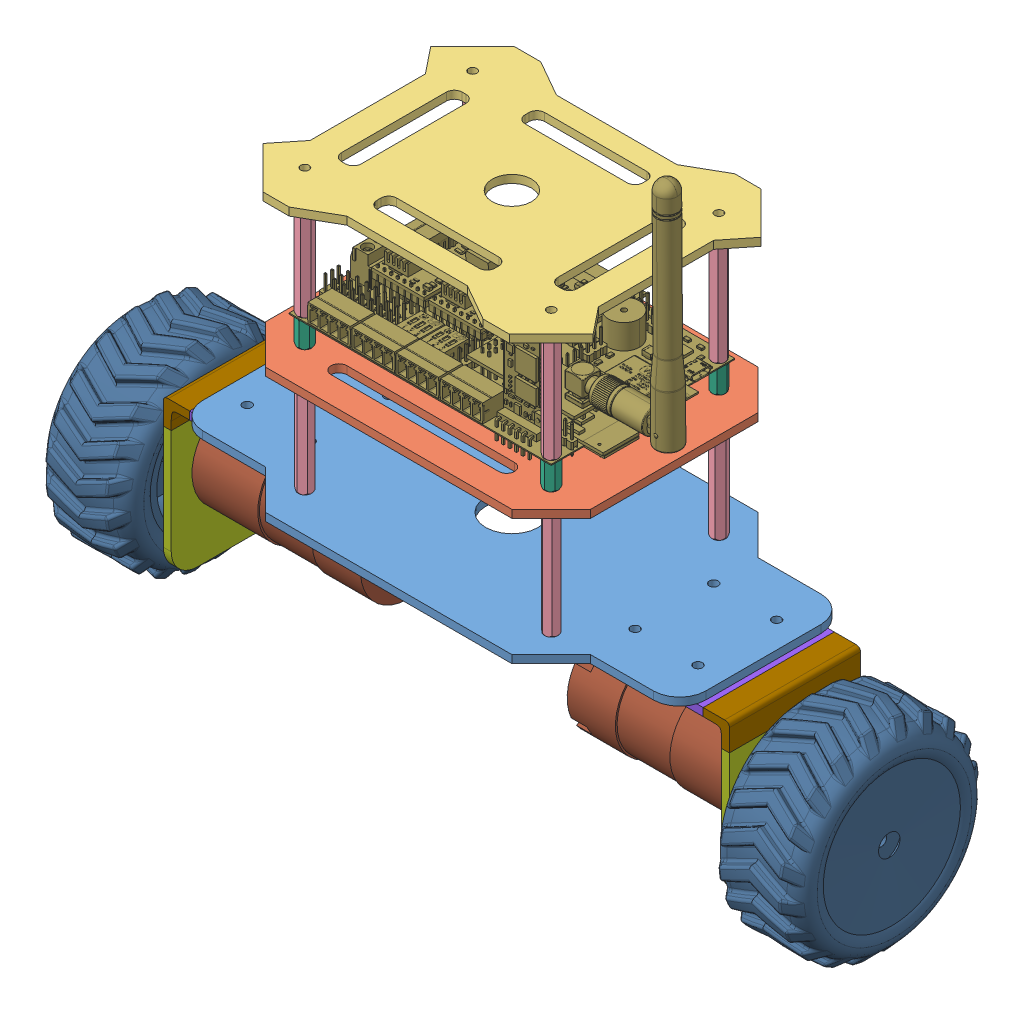
SolidWorks assembly Final, configuration Default. Lengths in mm.
Overall size (292 248.19 107.41).
32 component instances, 12 part files, 63 mates.
Components (placement in the parent):
- Part1-1: Part1 [Default] at (-40.5475 3 26.7241) x (1 0 0) z (0 -1 0) size (192 94 3)
- Part2-2: Part2 [Default] at (-62.5901 51 55.7188) x (1 0 0) z (0 -1 0) size (124 94 3)
- Part3-1: Part3 [Default] at (32.1399 109.4115 -37.8187) x (1 0 0) z (0 -1 0) size (126 96 3)
- MFM3L45mm^Final-1: MFM3L45mm^Final [Default] at (193.5375 3 45.3289) x (-0.984658 0 -0.174498) z (0 -1 0) size (5.02 6.48 51) (virtual)
- MFM3L45mm^Final-3: MFM3L45mm^Final [Default] at (9.2044 3 -151.3466) x (-0.509221 0 0.860636) z (0 -1 0) size (5.02 6.48 51) (virtual)
- MFM3L45mm^Final-4: MFM3L45mm^Final [Default] at (-148.574 3 -161.6746) x (0.815929 0 0.578152) z (0 -1 0) size (5.02 6.48 51) (virtual)
- MFM3L45mm^Final-5: MFM3L45mm^Final [Default] at (-34.8083 3 130.7081) x (-0.277574 0 -0.960704) z (0 -1 0) size (5.02 6.48 51) (virtual)
- MFM3L45mm^Final-6: MFM3L45mm^Final [Default] at (184.3979 61.4115 14.7735) x (-0.936555 0 -0.350522) z (0 -1 0) size (5.02 6.48 51) (virtual)
- MFM3L45mm^Final-7: MFM3L45mm^Final [Default] at (-232.6277 61.4115 -110.5112) x (0.76358 0 0.645713) z (0 -1 0) size (5.02 6.48 51) (virtual)
- MFM3L45mm^Final-8: MFM3L45mm^Final [Default] at (-70.3335 61.4115 137.3929) x (-0.0906 0 -0.995887) z (0 -1 0) size (5.02 6.48 51) (virtual)
- MFM3L45mm^Final-9: MFM3L45mm^Final [Default] at (-88.303 61.4115 176.86) x (0.498713 0 -0.866767) z (0 -1 0) size (5.02 6.48 51) (virtual)
- M3 Nut-2: M3 Nut [Default] at (-87.614 -1.2 -51.9559) x (0.520396 0 -0.853925) z (0 1 0) size (5.5 6.35 2.74)
- M3 Nut-3: M3 Nut [Default] at (-87.6542 -1.2 12.1323) x (-0.740225 0 0.672359) z (0 1 0) size (5.5 6.35 2.74)
- M3 Nut-4: M3 Nut [Default] at (6.4865 -1.2 12.0993) x (0.484551 0 0.874763) z (0 1 0) size (5.5 6.35 2.74)
- M3 Nut-6: M3 Nut [Default] at (6.3383 -1.2 -51.634) x (0.07396 0 0.997261) z (0 1 0) size (5.5 6.35 2.74)
- Hex Spacer MF M3 L10mm-1: Hex Spacer MF M3 L10mm [Default] at (-29.8707 51 -68.5775) x (0.908081 0 0.418795) z (0 -1 0) size (5.02 6.48 16)
- Hex Spacer MF M3 L10mm-2: Hex Spacer MF M3 L10mm [Default] at (-16.8725 51 -20.321) x (0.583126 0 0.812382) z (0 -1 0) size (5.02 6.48 16)
- Hex Spacer MF M3 L10mm-3: Hex Spacer MF M3 L10mm [Default] at (-50.7588 51 -36.1224) x (-0.919717 0 -0.392583) z (0 -1 0) size (5.02 6.48 16)
- Hex Spacer MF M3 L10mm-4: Hex Spacer MF M3 L10mm [Default] at (-74.6509 51 -25.6897) x (-0.322414 0 0.946599) z (0 -1 0) size (5.02 6.48 16)
- Assem2-3: Assem2 [Default] at (-95.5475 -21.4649 -20.3691) x (0 -1 0) z (-1 0 0) size (60 50 58)
  - Part5-1: Part5 [Default] at (12.5467 -0.7648 50) size (50 50 3)
  - Part4-1: Part4 [Default] at (-18.4649 10.92 18.3247) x (0 0 1) z (-1 0 0) size (48 50 3)
  - Part6-1: Part6 [Default] at (-13.4649 25.5434 24.5714) x (-1 0 0) z (0 -1 0) size (10 10 50)
- Assem2-4: Assem2 [Default] at (14.4525 -21.4649 -19.2823) x (0 -1 0) z (1 0 0) size (60 50 58)
  - Part5-1: Part5 [Default] at (12.5467 -0.7648 50) size (50 50 3)
  - Part4-1: Part4 [Default] at (-18.4649 10.92 18.3247) x (0 0 1) z (-1 0 0) size (48 50 3)
  - Part6-1: Part6 [Default] at (-13.4649 25.5434 24.5714) x (-1 0 0) z (0 -1 0) size (10 10 50)
- wheel-1: wheel [Default] at (-151.5475 -35 -19.8257) x (0 0.670753 0.741681) z (0 -0.741681 0.670753) size (76.03 35 76.06)
- wheel-2: wheel [Default] at (70.4525 -35 -19.8257) x (0 -0.773648 -0.633616) z (0 -0.633616 0.773648) size (76.03 35 76.06)
- Cytron Motor-1: Cytron Motor [Default] at (32.3025 -28.1657 -18.5629) x (0 0.5 -0.866025) z (0 0.866025 0.5) size (36.7 90.3 36.7)
- Cytron Motor-2: Cytron Motor [Default] at (-113.3975 -28.1657 -21.0886) x (0 0.5 0.866025) z (0 0.866025 -0.5) size (36.7 90.3 36.7)
- simple-1: simple [Default] at (-90.5475 61.4115 15.1743) x (1 0 0) z (0 1 0) size (131.96 75.31 110.74)
Mates (geometry in assembly coordinates):
- Coincident88: coincident anti-aligned: plane of Part1-1 through (-126.5475 0 2.1743) normal (0 -1 0)
- Concentric2: concentric anti-aligned: cylinder of Part1-1 through (-102.5475 0 -4.8257) axis (0 1 0) radius 1.7; cylinder of Assem2-3/Part4-1 through (-102.5475 0 -4.8257) axis (0 -1 0) radius 1.8145
- Coincident91: coincident anti-aligned: plane of Part1-1 through (-126.5475 0 2.1743) normal (0 -1 0); plane of Assem2-3/Part4-1 through (-100.5475 0 -34.8257) normal (0 1 0)
- Concentric3: concentric anti-aligned: cylinder of Part1-1 through (-126.5475 0 -34.8257) axis (0 1 0) radius 1.7; cylinder of Assem2-3/Part4-1 through (-126.5475 0 -34.8257) axis (0 -1 0) radius 1.873
- Concentric5: concentric anti-aligned: cylinder of Part1-1 through (21.4525 0 -4.8257) axis (0 1 0) radius 1.7; cylinder of Assem2-4/Part4-1 through (21.4525 0 -4.8257) axis (0 -1 0) radius 2.1419
- Concentric6: concentric anti-aligned: cylinder of Part1-1 through (45.4525 0 -34.8257) axis (0 1 0) radius 1.7; cylinder of Assem2-4/Part4-1 through (45.4525 0 -34.8257) axis (0 -1 0) radius 1.9958
- Coincident92: coincident anti-aligned: plane of Part1-1 through (-126.5475 0 2.1743) normal (0 -1 0); plane of Assem2-4/Part4-1 through (19.4525 0 -4.8257) normal (0 1 0)
- Coincident101: coincident anti-aligned: plane of Part1-1 through (-126.5475 3 2.1743) normal (0 1 0); plane of MFM3L45mm^Final-4 through (5.8462 3 -55.3806) normal (0 -1 0)
- Concentric9: concentric anti-aligned: cylinder of Part1-1 through (6.4525 0 -51.8257) axis (0 1 0) radius 1.7; cylinder of MFM3L45mm^Final-4 through (6.4525 47.7566 -51.8257) axis (0 -1 0) radius 1.2
- Coincident103: coincident anti-aligned: plane of Part1-1 through (-126.5475 3 2.1743) normal (0 1 0); plane of MFM3L45mm^Final-1 through (8.5184 3 15.1301) normal (0 -1 0)
- Coincident104: coincident anti-aligned: plane of Part1-1 through (-126.5475 3 2.1743) normal (0 1 0); plane of MFM3L45mm^Final-5 through (-89.2894 3 -48.6681) normal (0 -1 0)
- Concentric11: concentric anti-aligned: cylinder of Part1-1 through (-87.5475 0 -51.8257) axis (0 1 0) radius 1.7; cylinder of MFM3L45mm^Final-5 through (-87.5475 47.7566 -51.8257) axis (0 -1 0) radius 1.2
- Coincident105: coincident anti-aligned: plane of Part1-1 through (-126.5475 3 2.1743) normal (0 1 0); plane of MFM3L45mm^Final-3 through (-84.0543 3 11.2782) normal (0 -1 0)
- Concentric12: concentric anti-aligned: cylinder of Part1-1 through (-87.5475 0 12.1743) axis (0 1 0) radius 1.7; cylinder of MFM3L45mm^Final-3 through (-87.5475 47.7566 12.1743) axis (0 -1 0) radius 1.2
- Coincident106: coincident anti-aligned: plane of Part1-1 through (-126.5475 0 2.1743) normal (0 -1 0); plane of M3 Nut-4 through (6.4865 0 12.0993) normal (0 1 0)
- Coincident110: coincident anti-aligned: plane of Part1-1 through (-126.5475 0 2.1743) normal (0 -1 0); plane of M3 Nut-4 through (6.4865 0 12.0993) normal (0 1 0)
- Coincident111: coincident anti-aligned: plane of Part1-1 through (-126.5475 0 2.1743) normal (0 -1 0); plane of M3 Nut-4 through (6.4865 0 12.0993) normal (0 1 0)
- Lock2: lock: unknown of MFM3L45mm^Final-1; unknown of M3 Nut-4
- Coincident112: coincident anti-aligned: plane of Part1-1 through (-126.5475 0 2.1743) normal (0 -1 0); plane of M3 Nut-3 through (-87.6542 0 12.1323) normal (0 1 0)
- Lock3: lock: unknown of MFM3L45mm^Final-3; unknown of M3 Nut-3
- Coincident113: coincident anti-aligned: plane of Part1-1 through (-126.5475 0 2.1743) normal (0 -1 0); plane of M3 Nut-6 through (6.3383 0 -51.634) normal (0 1 0)
- Lock5: lock: unknown of MFM3L45mm^Final-4; unknown of M3 Nut-6
- Coincident115: coincident anti-aligned: plane of Part1-1 through (-126.5475 0 2.1743) normal (0 -1 0); plane of M3 Nut-2 through (-87.614 0 -51.9559) normal (0 1 0)
- Concentric13: concentric anti-aligned: cylinder of Part2-2 through (6.4525 48 12.1743) axis (0 1 0) radius 1.8; cylinder of MFM3L45mm^Final-1 through (6.4525 47.7566 12.1743) axis (0 -1 0) radius 1.2
- Coincident116: coincident anti-aligned: plane of Part2-2 through (-62.5901 48 55.7188) normal (0 -1 0); plane of MFM3L45mm^Final-1 through (8.5184 48 15.1301) normal (0 1 0)
- Concentric14: concentric anti-aligned: cylinder of Part2-2 through (-87.5475 48 -51.8257) axis (0 1 0) radius 1.8; cylinder of MFM3L45mm^Final-5 through (-87.5475 47.7566 -51.8257) axis (0 -1 0) radius 1.2
- Coincident117: coincident anti-aligned: plane of Part2-2 through (-62.5901 51 55.7188) normal (0 1 0); plane of Hex Spacer MF M3 L10mm-2 through (7.0371 51 8.6157) normal (0 -1 0)
- Coincident118: coincident anti-aligned: plane of Part2-2 through (-62.5901 51 55.7188) normal (0 1 0); plane of Hex Spacer MF M3 L10mm-3 through (-86.2033 51 -48.4794) normal (0 -1 0)
- Concentric16: concentric aligned: cylinder of Part2-2 through (-87.5475 48 -51.8257) axis (0 1 0) radius 1.8; cylinder of Hex Spacer MF M3 L10mm-3 through (-87.5475 54.7566 -51.8257) axis (0 1 0) radius 1.2
- Coincident120: coincident anti-aligned: plane of Part2-2 through (-62.5901 51 55.7188) normal (0 1 0); plane of Hex Spacer MF M3 L10mm-1 through (5.2049 51 -55.2092) normal (0 -1 0)
- Concentric17: concentric aligned: cylinder of Part2-2 through (6.4525 48 -51.8257) axis (0 1 0) radius 1.8; cylinder of Hex Spacer MF M3 L10mm-1 through (6.4525 54.7566 -51.8257) axis (0 1 0) radius 1.2
- Coincident121: coincident anti-aligned: plane of Part2-2 through (-62.5901 51 55.7188) normal (0 1 0); plane of Hex Spacer MF M3 L10mm-4 through (-84.3115 51 10.5826) normal (0 -1 0)
- Concentric18: concentric aligned: cylinder of Part2-2 through (-87.5475 48 12.1743) axis (0 1 0) radius 1.8; cylinder of Hex Spacer MF M3 L10mm-4 through (-87.5475 54.7566 12.1743) axis (0 1 0) radius 1.2
- Concentric25: concentric anti-aligned: cylinder of Part3-1 through (-87.5475 106.4115 -51.8257) axis (0 1 0) radius 1.6; cylinder of MFM3L45mm^Final-8 through (-87.5475 106.1681 -51.8257) axis (0 -1 0) radius 1.2
- Lock6: lock: unknown of MFM3L45mm^Final-5; unknown of M3 Nut-2
- Coincident129: coincident anti-aligned: plane of Assem2-4/Part5-1 through (64.4525 -50 -4.8257) normal (-1 0 0); plane of Cytron Motor-1 through (64.4525 -18.9907 -34.4544) normal (1 0 0)
- Concentric27: concentric aligned: cylinder of Assem2-4/Part5-1 through (67.4525 -35 -19.8257) axis (-1 0 0) radius 5; cylinder of Cytron Motor-1 through (70.4525 -35 -19.8257) axis (-1 0 0) radius 5.95
- Coincident130: coincident anti-aligned: plane of Assem2-3/Part5-1 through (-145.5475 -50 -34.8257) normal (1 0 0); plane of Cytron Motor-2 through (-145.5475 -18.9907 -5.197) normal (-1 0 0)
- Concentric28: concentric aligned: cylinder of Assem2-3/Part5-1 through (-148.5475 -35 -19.8257) axis (1 0 0) radius 5; cylinder of Cytron Motor-2 through (-151.5475 -35 -19.8257) axis (1 0 0) radius 5.95
- Coincident132: coincident anti-aligned: plane of Assem2-3/Part5-1 through (-145.5475 -50 -34.8257) normal (1 0 0); plane of Cytron Motor-2 through (-145.5475 -18.9907 -5.197) normal (-1 0 0)
- Parallel2: parallel anti-aligned: plane of Assem2-3/Part4-1 through (-100.5475 -3 -34.8257) normal (0 -1 0); plane of Cytron Motor-2 through (-87.2475 -18.1386 -21.0886) normal (0 1 0)
- Parallel3: parallel anti-aligned: plane of Part1-1 through (-126.5475 0 2.1743) normal (0 -1 0); plane of Cytron Motor-1 through (6.1525 -18.1386 -18.5629) normal (0 1 0)
- Concentric29: concentric anti-aligned: circle of wheel-1; circle of Cytron Motor-2
- Concentric30: concentric anti-aligned: circle of wheel-2; circle of Cytron Motor-1
- Coincident137: coincident anti-aligned: plane of wheel-2 through (90.4525 -35 -19.8257) normal (-1 0 0); plane of Cytron Motor-1 through (90.4525 -35 -19.8257) normal (1 0 0)
- Coincident138: coincident anti-aligned: plane of wheel-1 through (-171.5475 -35 -19.8257) normal (1 0 0); plane of Cytron Motor-2 through (-171.5475 -35 -19.8257) normal (-1 0 0)
- Concentric32: concentric anti-aligned: cylinder of Part1-1 through (6.4525 0 12.1743) axis (0 1 0) radius 1.7; cylinder of MFM3L45mm^Final-1 through (6.4525 47.7566 12.1743) axis (0 -1 0) radius 1.2
- Concentric33: concentric aligned: cylinder of Part2-2 through (6.4525 48 12.1743) axis (0 1 0) radius 1.8; cylinder of Hex Spacer MF M3 L10mm-2 through (6.4525 54.7566 12.1743) axis (0 1 0) radius 1.2
- Parallel4: parallel anti-aligned: plane of Part2-2 through (-62.5901 51 55.7188) normal (0 1 0); plane of simple-1 through (-90.5475 61 15.1743) normal (0 -1 0)
- Concentric34: concentric anti-aligned: cylinder of Hex Spacer MF M3 L10mm-1 through (6.4525 54.7566 -51.8257) axis (0 1 0) radius 1.2; cylinder of simple-1 through (6.4525 61 -51.8257) axis (0 -1 0) radius 1.5
- Coincident140: coincident anti-aligned: plane of Hex Spacer MF M3 L10mm-1 through (5.2049 61 -55.2092) normal (0 1 0); plane of simple-1 through (-90.5475 61 15.1743) normal (0 -1 0)
- Concentric35: concentric anti-aligned: cylinder of Hex Spacer MF M3 L10mm-4 through (-87.5475 54.7566 12.1743) axis (0 1 0) radius 1.2; cylinder of simple-1 through (-87.5475 61 12.1743) axis (0 -1 0) radius 1.5
- Concentric36: concentric anti-aligned: cylinder of MFM3L45mm^Final-8 through (-87.5475 106.1681 -51.8257) axis (0 -1 0) radius 1.2; cylinder of Hex Spacer MF M3 L10mm-3 through (-87.5475 54.7566 -51.8257) axis (0 1 0) radius 1.2
- Coincident141: coincident anti-aligned: plane of MFM3L45mm^Final-8 through (-89.8559 61.4115 -49.0552) normal (0 -1 0); plane of simple-1 through (-90.5475 61.4115 15.1743) normal (0 1 0)
- Coincident142: coincident anti-aligned: plane of MFM3L45mm^Final-6 through (7.9469 61.4115 -48.5437) normal (0 -1 0); plane of simple-1 through (-90.5475 61.4115 15.1743) normal (0 1 0)
- Concentric37: concentric anti-aligned: cylinder of MFM3L45mm^Final-6 through (6.4525 106.1681 -51.8257) axis (0 -1 0) radius 1.2; cylinder of Hex Spacer MF M3 L10mm-1 through (6.4525 54.7566 -51.8257) axis (0 1 0) radius 1.2
- Coincident143: coincident anti-aligned: plane of MFM3L45mm^Final-7 through (-87.848 61.4115 8.5806) normal (0 -1 0); plane of simple-1 through (-90.5475 61.4115 15.1743) normal (0 1 0)
- Concentric38: concentric anti-aligned: cylinder of MFM3L45mm^Final-7 through (-87.5475 106.1681 12.1743) axis (0 -1 0) radius 1.2; cylinder of Hex Spacer MF M3 L10mm-4 through (-87.5475 54.7566 12.1743) axis (0 1 0) radius 1.2
- Coincident144: coincident anti-aligned: plane of MFM3L45mm^Final-9 through (2.9706 61.4115 13.1128) normal (0 -1 0); plane of simple-1 through (-90.5475 61.4115 15.1743) normal (0 1 0)
- Concentric41: concentric anti-aligned: cylinder of MFM3L45mm^Final-9 through (6.4525 106.1681 12.1743) axis (0 -1 0) radius 1.2; cylinder of Hex Spacer MF M3 L10mm-2 through (6.4525 54.7566 12.1743) axis (0 1 0) radius 1.2
- Concentric42: concentric anti-aligned: cylinder of Part3-1 through (-87.5475 106.4115 -51.8257) axis (0 1 0) radius 1.6; cylinder of MFM3L45mm^Final-8 through (-87.5475 106.1681 -51.8257) axis (0 -1 0) radius 1.2
- Coincident145: coincident anti-aligned: plane of Part3-1 through (32.1399 106.4115 -37.8187) normal (0 -1 0); plane of MFM3L45mm^Final-8 through (-89.8559 106.4115 -49.0552) normal (0 1 0)
- Concentric43: concentric anti-aligned: cylinder of Part3-1 through (6.4525 106.4115 12.1743) axis (0 1 0) radius 1.6; cylinder of MFM3L45mm^Final-9 through (6.4525 106.1681 12.1743) axis (0 -1 0) radius 1.2
